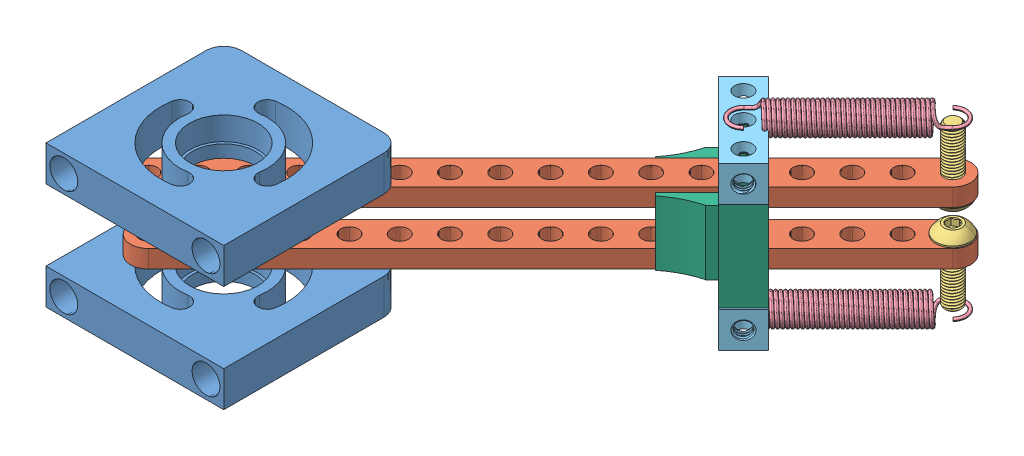
SolidWorks assembly Drone Launcher Assembly, configuration Default. Lengths in mm.
Overall size (105.44 43.78 109.92).
17 component instances, 8 part files, 40 mates.
Components (placement in the parent):
- Drone Launcher Base-1: Drone Launcher Base [Default] at (9.5832 21.5969 33.0344) size (46.27 8 60.08)
- Drone Launcher Base-2: Drone Launcher Base [Default] at (9.5832 45.5969 33.0344) size (46.27 8 60.08)
- 17 hole flat beam.step-1: 17 hole flat beam.step [Default] at (44.1155 29.5969 -5.9724) x (0.707107 0 -0.707107) z (0.707107 0 0.707107) size (136 4 8)
- 17 hole flat beam.step-2: 17 hole flat beam.step [Default] at (44.1155 41.5969 -5.9724) x (0.707107 0 -0.707107) z (0.707107 0 0.707107) size (136 4 8)
- 14mm button head screw.step-1: 14mm button head screw.step [Default] at (89.3704 39.3969 -51.2272) x (0.997884 0 -0.065013) z (0 -1 0) size (7.6 7.6 16.21)
- 14mm button head screw.step-2: 14mm button head screw.step [Default] at (89.3704 35.7969 -51.2272) x (-0.454677 0 -0.890656) z (0 1 0) size (7.6 7.6 16.21)
- 90404S.stp-1: 90404S.stp [Default] at (77.5883 18.9607 -39.4451) x (0.707107 0 -0.707107) z (-0.707107 0 -0.707107) size (39.64 6.51 6.51)
  - EXTENSION.stp-1: EXTENSION.stp [Default] at origin size (39.64 6.51 6.51)
- 90404S.stp-3: 90404S.stp [Default] at (77.5883 56.233 -39.4451) x (0.707107 0 -0.707107) z (0.707107 0 0.707107) size (39.64 6.51 6.51)
  - EXTENSION.stp-1: EXTENSION.stp [Default] at origin size (39.64 6.51 6.51)
- lock nut.step-1: lock nut.step [Default] at (89.3704 18.5946 -51.2272) x (0.258819 0 -0.965926) z (-0.965926 0 -0.258819) (suppressed, hidden)
- 3 hole square beam.step-1: 3 hole square beam.step [Default] at (60.1493 23.3426 -33.3198) x (0.707107 0 -0.707107) z (0 -1 0) size (8 24.01 8)
- 3 hole square beam.step-3: 3 hole square beam.step [Default] at (60.1493 51.8511 -33.3198) x (-0.707107 0 0.707107) z (0 1 0) size (8 24.01 8)
- New Bracket-1: New Bracket [Default] at (68.6346 37.5926 -30.4914) x (0 -1 0) z (-0.707107 0 -0.707107) size (20.5 18 23.2)
- Spacer For Spring Launcher-1: Spacer For Spring Launcher [Default] at (89.3704 19.3269 -51.2272) x (0.980554 0 0.196247) z (-0.196247 0 0.980554) (suppressed, hidden)
- Spacer For Spring Launcher-2: Spacer For Spring Launcher [Default] at (89.3704 45.5969 -51.2272) x (0.996904 0 0.078631) z (-0.078631 0 0.996904) (suppressed, hidden)
- lock nut.step-2: lock nut.step [Default] at (89.3704 56.5991 -51.2272) x (0.707107 0 0.707107) z (-0.707107 0 0.707107) (suppressed, hidden)
Mates (geometry in assembly coordinates):
- Coincident1: coincident aligned: plane of Drone Launcher Base-1 through (-10.4168 29.5969 53.0344) normal (-1 0 0); plane of Drone Launcher Base-2 through (-10.4168 53.5969 53.0344) normal (-1 0 0)
- Coincident2: coincident aligned: plane of Drone Launcher Base-1 through (-10.4168 29.5969 53.0344) normal (0 0 1); plane of Drone Launcher Base-2 through (-10.4168 53.5969 53.0344) normal (0 0 1)
- Coincident5: coincident anti-aligned: plane of Drone Launcher Base-1 through (9.5832 29.5969 33.0344) normal (0 1 0); plane of 17 hole flat beam.step-1 through (-1.1393 29.5969 39.2825) normal (0 -1 0)
- Parallel3: parallel aligned: plane of 17 hole flat beam.step-1 through (-3.9677 33.5969 36.4541) normal (-0.707107 0 -0.707107); plane of 17 hole flat beam.step-2 through (-3.9677 45.5969 36.4541) normal (-0.707107 0 -0.707107)
- Coincident7: coincident anti-aligned: plane of Drone Launcher Base-2 through (9.5832 45.5969 33.0344) normal (0 -1 0); plane of 17 hole flat beam.step-2 through (-1.1393 45.5969 39.2825) normal (0 1 0)
- Coincident8: coincident aligned: plane of 17 hole flat beam.step-1 through (-3.9677 33.5969 36.4541) normal (-0.707107 0 -0.707107); plane of 17 hole flat beam.step-2 through (-3.9677 45.5969 36.4541) normal (-0.707107 0 -0.707107)
- Concentric8: concentric aligned: cylinder of 17 hole flat beam.step-1 through (-1.1393 33.5969 39.2825) axis (0 1 0) radius 2; cylinder of 17 hole flat beam.step-2 through (-1.1393 45.5969 39.2825) axis (0 1 0) radius 2
- Tangent5: tangent aligned: cylinder of Drone Launcher Base-2 through (9.5832 53.5969 33.0344) axis (0 -1 0) radius 7.1; cylinder of 17 hole flat beam.step-2 through (4.5176 45.5969 33.6256) axis (0 1 0) radius 2
- Tangent6: tangent aligned: cylinder of Drone Launcher Base-2 through (9.5832 53.5969 33.0344) axis (0 -1 0) radius 7.1; cylinder of 17 hole flat beam.step-2 through (10.1744 45.5969 27.9688) axis (0 1 0) radius 2
- Distance2: distance = 24 mm: cylinder of Drone Launcher Base-1 through (-6.4168 25.5969 48.3344) axis (0 0 1) radius 3.15; cylinder of Drone Launcher Base-2 through (-6.4168 49.5969 48.3344) axis (0 0 1) radius 3.15
- Angle2: planar angle = 2.356194 rad anti-aligned: plane of 17 hole flat beam.step-2 through (-3.9677 45.5969 36.4541) normal (-0.707107 0 -0.707107); plane of Drone Launcher Base-2 through (-10.4168 53.5969 13.0344) normal (0 0 -1)
- Concentric12: concentric anti-aligned: cylinder of 17 hole flat beam.step-1 through (89.3704 33.5969 -51.2272) axis (0 1 0) radius 2; circle of 14mm button head screw.step-1
- Coincident10: coincident anti-aligned: plane of 17 hole flat beam.step-2 through (-1.1393 41.5969 39.2825) normal (0 -1 0); plane of 14mm button head screw.step-1 through (89.1233 41.5969 -55.0191) normal (0 1 0)
- Concentric13: concentric aligned: cylinder of 17 hole flat beam.step-1 through (89.3704 33.5969 -51.2272) axis (0 1 0) radius 2; circle of 14mm button head screw.step-2
- Coincident11: coincident anti-aligned: plane of 17 hole flat beam.step-1 through (-1.1393 33.5969 39.2825) normal (0 1 0); plane of 14mm button head screw.step-2 through (92.7549 33.5969 -52.955) normal (0 -1 0)
- Concentric23: concentric anti-aligned: circle of 90404S.stp-1/EXTENSION.stp-1; circle of 90404S.stp-3/EXTENSION.stp-1
- Tangent10: tangent anti-aligned: torus of 90404S.stp-1/EXTENSION.stp-1; plane of lock nut.step-1 through (93.2741 18.5946 -50.1812) normal (0 1 0)
- Coincident26: coincident aligned: plane of 3 hole square beam.step-1 through (57.3209 23.3426 -36.1483) normal (-0.707107 0 -0.707107); plane of 3 hole square beam.step-3 through (57.3209 51.8511 -36.1483) normal (-0.707107 0 -0.707107)
- Parallel7: parallel aligned: plane of 17 hole flat beam.step-1 through (-3.9677 33.5969 36.4541) normal (-0.707107 0 -0.707107); plane of 3 hole square beam.step-1 through (57.3209 23.3426 -36.1483) normal (-0.707107 0 -0.707107)
- Coincident29: coincident aligned: plane of 3 hole square beam.step-1 through (60.1493 23.3426 -27.663) normal (-0.707107 0 0.707107); plane of 3 hole square beam.step-3 through (60.1493 51.8511 -27.663) normal (-0.707107 0 0.707107)
- Concentric26: concentric anti-aligned: circle of 90404S.stp-1/EXTENSION.stp-1; cylinder of 3 hole square beam.step-1 through (65.8062 27.3426 -27.663) axis (0 1 0) radius 2
- Tangent11: tangent anti-aligned: torus of 90404S.stp-1/EXTENSION.stp-1; plane of 3 hole square beam.step-1 through (62.9778 19.3426 -30.4914) normal (0 -1 0)
- Concentric27: concentric anti-aligned: circle of 17 hole flat beam.step-1; circle of 90404S.stp-1/EXTENSION.stp-1
- Concentric28: concentric anti-aligned: circle of 17 hole flat beam.step-1; cylinder of Spacer For Spring Launcher-1 through (89.3704 29.5969 -51.2272) axis (0 -1 0) radius 3.8
- Tangent12: tangent anti-aligned: torus of 90404S.stp-1/EXTENSION.stp-1; plane of Spacer For Spring Launcher-1 through (89.3704 19.3269 -51.2272) normal (0 -1 0)
- Concentric29: concentric anti-aligned: circle of 17 hole flat beam.step-2; cylinder of Spacer For Spring Launcher-2 through (89.3704 55.8669 -51.2272) axis (0 -1 0) radius 3.8
- Concentric30: concentric anti-aligned: circle of 90404S.stp-3/EXTENSION.stp-1; cylinder of Spacer For Spring Launcher-2 through (89.3704 55.8669 -51.2272) axis (0 -1 0) radius 3.8
- Tangent14: tangent anti-aligned: torus of 90404S.stp-3/EXTENSION.stp-1; plane of Spacer For Spring Launcher-2 through (89.3704 55.8669 -51.2272) normal (0 1 0)
- Coincident37: coincident anti-aligned: plane of 17 hole flat beam.step-2 through (-1.1393 45.5969 39.2825) normal (0 1 0); plane of Spacer For Spring Launcher-2 through (89.3704 45.5969 -51.2272) normal (0 -1 0)
- Tangent15: tangent anti-aligned: torus of 90404S.stp-3/EXTENSION.stp-1; plane of lock nut.step-2 through (92.2281 56.5991 -54.0849) normal (0 -1 0)
- Concentric31: concentric aligned: circle of lock nut.step-1; cylinder of Spacer For Spring Launcher-1 through (89.3704 29.5969 -51.2272) axis (0 -1 0) radius 3.8
- Concentric32: concentric aligned: cylinder of Spacer For Spring Launcher-2 through (89.3704 55.8669 -51.2272) axis (0 -1 0) radius 3.8; circle of lock nut.step-2
- Coincident38: coincident aligned: plane of lock nut.step-1 through (85.4666 13.7446 -52.2732) normal (-0.707107 0 -0.707107); plane of lock nut.step-2 through (88.3244 61.4491 -55.1309) normal (-0.707107 0 -0.707107)
- Parallel8: parallel aligned: plane of 17 hole flat beam.step-2 through (-3.9677 45.5969 36.4541) normal (-0.707107 0 -0.707107); plane of lock nut.step-2 through (88.3244 61.4491 -55.1309) normal (-0.707107 0 -0.707107)
- Coincident39: coincident anti-aligned: plane of 17 hole flat beam.step-1 through (-1.1393 29.5969 39.2825) normal (0 -1 0); circle of Spacer For Spring Launcher-1
- Coincident40: coincident anti-aligned: plane of 3 hole square beam.step-1 through (62.9778 27.3426 -30.4914) normal (0 1 0); plane of New Bracket-1 through (66.089 27.3426 -21.7233) normal (0 -1 0)
- Tangent16: tangent anti-aligned: torus of 90404S.stp-3/EXTENSION.stp-1; plane of 3 hole square beam.step-3 through (62.9778 55.8511 -30.4914) normal (0 1 0)
- Parallel9: parallel: line of 17 hole flat beam.step-1; line of 90404S.stp-1/EXTENSION.stp-1 through (86.155 18.9607 -52.463) axis (0.707107 0 -0.707107)
- Concentric33: concentric aligned: cylinder of 3 hole square beam.step-3 through (60.1493 47.8511 -33.3198) axis (0 -1 0) radius 2; cylinder of New Bracket-1 through (60.1493 48.0426 -33.3198) axis (0 -1 0) radius 2.1
- Concentric34: concentric aligned: cylinder of 3 hole square beam.step-3 through (71.463 47.8511 -22.0061) axis (0 -1 0) radius 2; cylinder of New Bracket-1 through (71.463 48.0426 -22.0061) axis (0 -1 0) radius 2.1
